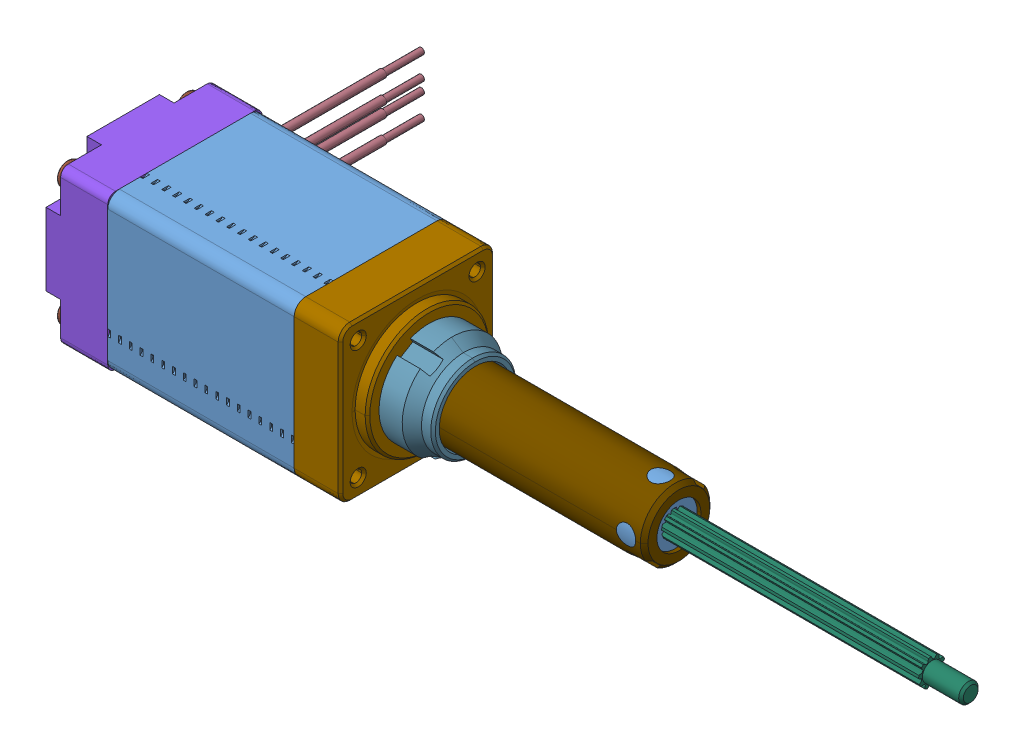
SolidWorks assembly 20NC38..31, configuration 默认. Lengths in mm.
Overall size (109.8 25.88 45.74).
31 component instances, 19 part files, 0 mates.
Components (placement in the parent):
- 20NC38..31.STEP-1: 20NC38..31.STEP [默认] at origin size (109.8 25.88 45.74)
  - 02-20-38.15________.STEP-1: 02-20-38.15________.STEP [默认] at origin size (39.65 25.88 45.74)
    - 02-20-38.STEP-1: 02-20-38.STEP [默认] at (20.075 0 0) x (0 0 1) z (-1 0 0) size (26.04 25.88 31.46)
      - 02-20-24.15_10-20-001-2.STEP-1: 02-20-24.15_10-20-001-2.STEP [默认] at origin size (20 20 24.15)
      - 13-20-8.5____.STEP-1: 13-20-8.5____.STEP [默认] at (0 0 16.075) x (0 1 0) z (0 0 -1) size (18.2 22.2 10.51)
      - 13-20-12.5______.STEP-1: 13-20-12.5______.STEP [默认] at (0 0 -14.575) x (0.707107 0.707107 0) z (0 0 1) size (18.3 18.3 15.8)
    - 03-20-008______38_______default.STEP-1: 03-20-008______38_______default.STEP [默认] at (3.8 0 0) x (1 0 0) z (0 0.78069 0.624918) size (32.3 16.26 16.27)
      - 06-20-008______38_________01-20-007-1.STEP-1: 06-20-008______38_________01-20-007-1.STEP [默认] at origin size (32.3 7 7)
      - 03-20-4.2-6YK_10-20-006-2.STEP-1: 03-20-4.2-6YK_10-20-006-2.STEP [默认] at (24.2 0 0) x (0 0.91534 0.402682) z (-1 0 0) size (12.06 12.08 4.24)
      - 10-20-001__________.STEP-1: 10-20-001__________.STEP [默认] at (16.9 0 0) x (0 0 1) z (-1 0 0) size (11 11 1)
      - 08-20-001______1_______07-20-001-1.STEP-1: 08-20-001______1_______07-20-001-1.STEP [默认] at (22.1 0 0) x (0 0 1) z (-1 0 0) size (11 11 1)
      - 08-20-001______1_______07-20-001-1.STEP-2: 08-20-001______1_______07-20-001-1.STEP [默认] at (11.4 0 0) x (0 0 1) z (-1 0 0) size (11 11 1)
      - 03-20-4.2-6YK_10-20-006-2.STEP-2: 03-20-4.2-6YK_10-20-006-2.STEP [默认] at (19 0 0) x (0 0.888249 0.459362) z (-1 0 0) size (12.06 12.08 4.24)
      - 03-20-4.2-6YK_10-20-006-2.STEP-3: 03-20-4.2-6YK_10-20-006-2.STEP [默认] at (13.5 0 0) x (0 0.91534 0.402682) z (-1 0 0) size (12.06 12.08 4.24)
      - 03-20-4.2-6YK_10-20-006-2.STEP-4: 03-20-4.2-6YK_10-20-006-2.STEP [默认] at (8.3 0 0) x (0 0.888249 0.459362) z (-1 0 0) size (12.06 12.08 4.24)
    - 01-20-003__20__________________.STEP-1: 01-20-003__20__________________.STEP [默认] at origin size (8.8 20 20)
    - 01-20-001__20__________________.STEP-1: 01-20-001__20__________________.STEP [默认] at (31.35 0 0) x (0 0 1) z (1 0 0) size (20 20 8.3)
    - 09-20-001____9X__5X4)_09-20-001.STEP-1: 09-20-001____9X__5X4)_09-20-001.STEP [默认] at (33.1 0 0) x (1 0 0) z (0 0.994502 0.104719) size (3 9 9)
    - 09-20-001____9X__5X4)_09-20-001.STEP-2: 09-20-001____9X__5X4)_09-20-001.STEP [默认] at (3.8 0 0) x (1 0 0) z (0 -0.49427 -0.869308) size (3 9 9)
    - 11-20-002__M2-37__20-42__.STEP-1: 11-20-002__M2-37__20-42__.STEP [默认] at (0.39 -7.7 7.7) x (0 0 -1) z (1 0 0) size (3 3 33)
    - 11-20-002__M2-37__20-42__.STEP-2: 11-20-002__M2-37__20-42__.STEP [默认] at (0.39 -7.7 -7.7) x (0 1 0) z (1 0 0) size (3 3 33)
    - 11-20-002__M2-37__20-42__.STEP-3: 11-20-002__M2-37__20-42__.STEP [默认] at (0.39 7.7 -7.7) x (0 0 1) z (1 0 0) size (3 3 33)
    - 11-20-002__M2-37__20-42__.STEP-4: 11-20-002__M2-37__20-42__.STEP [默认] at (0.39 7.7 7.7) x (0 -1 0) z (1 0 0) size (3 3 33)
    - 06-20-099__20___________20____________YK.STEP-1: 06-20-099__20___________20____________YK.STEP [默认] at (31.1 0 0) x (0 -0.624918 0.78069) z (-1 0 0) size (6.01 6.01 10)
    - 14-20-001__20-28____________________.STEP-1: 14-20-001__20-28____________________.STEP [默认] at (6.15 0 -8.6) x (0 -1 0) z (0 0 1) size (10.5 3.4 24.5)
  - 07-20-007__________________.STEP-1: 07-20-007__________________.STEP [默认] at (39.65 0 0) x (-1 0 0) z (0 -0.999857 -0.016895) size (6 12.92 13)
  - 07-20-013-2______________.STEP-1: 07-20-013-2______________.STEP [默认] at (68.4 0 0) x (0 -0.714016 0.700129) z (1 0 0) size (3.42 3.5 41.4)
  - 07-20-013-3______________.STEP-1: 07-20-013-3______________.STEP [默认] at (20.15 0 0) x (0 0.924225 0.381849) z (1 0 0) size (8 8 56.63)
  - 07-20-006__20______.STEP-1: 07-20-006__20______.STEP [默认] at (67.9 0 0) x (0 0.924225 0.381849) z (1 0 0) size (3.9 4.45 0.4)
  - 07-20-013-1__20_____________08-20-002-1.STEP-1: 07-20-013-1__20_____________08-20-002-1.STEP [默认] at (36.1 0 0) x (0 0.004204 -0.999991) z (1 0 0) size (9.01 9.01 35.91)
  - 07-20-002__20________________.STEP-1: 07-20-002__20________________.STEP [默认] at (69.65 0 0) x (0 0.004204 -0.999991) z (1 0 0) size (9.01 9.01 3.1)
